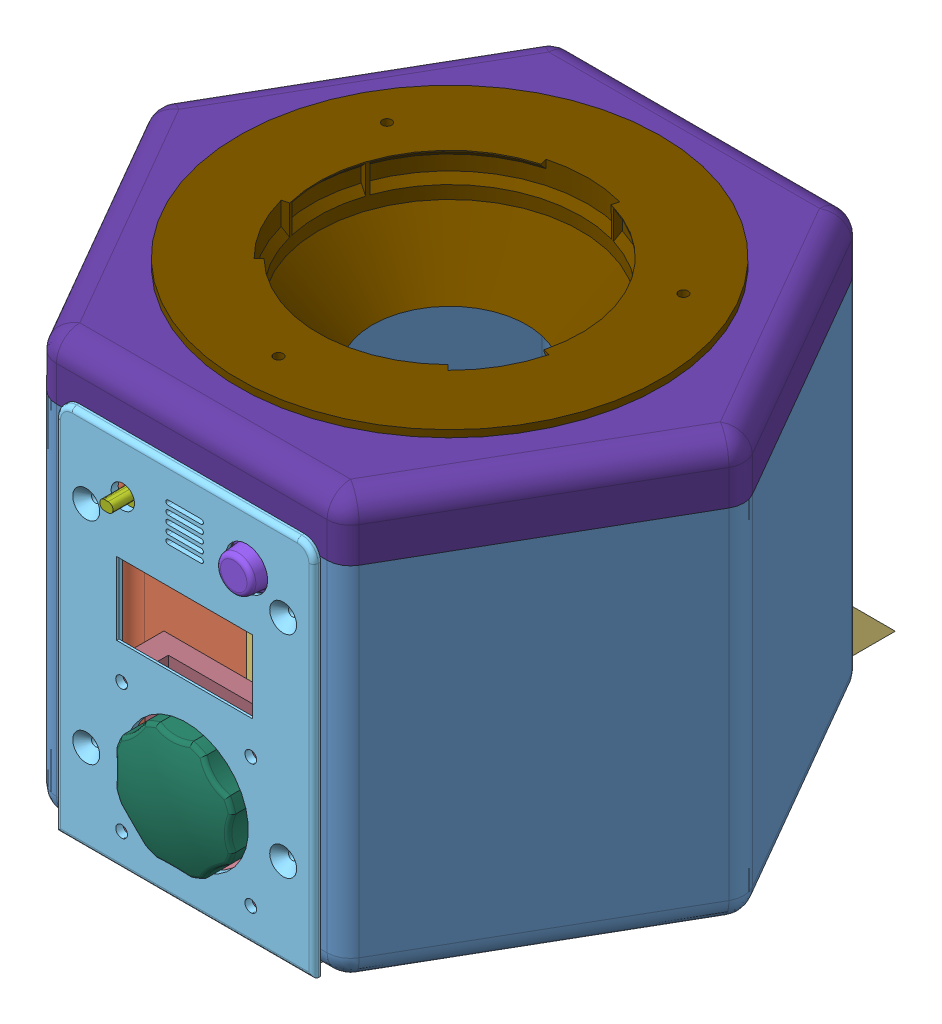
SolidWorks assembly Assy_base_tanque, configuration Default. Lengths in mm.
Overall size (250.94 210.12 285.79).
23 component instances, 18 part files, 9 mates.
Components (placement in the parent):
- base  1_1-1: base  1_1 [Default] at (121.3241 94.324 202.911) size (250.94 155 220)
- Assy_box_control-1: Assy_box_control [Default] at (251.8598 45.2792 -150.6249) size (110 187.12 285.79)
  - box-control_D-1: box-control_D [Default] at (-180.6357 49.0448 463.5359) size (50.1 155 250)
  - box-control_I-1: box-control_I [Default] at (-82.0357 49.0448 463.5359) size (50.1 155 250)
  - base_control_box-1: base_control_box [Default] at (-178.5357 49.0448 465.1037) size (96 25 220)
  - frente_control_box-1: frente_control_box [Default] at (-185.5357 49.0448 463.5359) size (110 160 8.5)
  - DS3231 RTC-2: DS3231 RTC [Default] at (-98.9357 55.5448 310.9359) x (0 0 -1) z (0 -1 0) size (44.75 22.8 13.53)
    - Default-1: Default [Predeterminado] at origin size (44.75 22.8 13.53)
  - LDR-1: LDR [Default] at (-156.876 173.9735 458.6019) x (1 0 0) z (0 0 -1) size (14.2 40.8 21.6)
  - MQ135_sensor-1: MQ135_sensor [Default] at (-98.6357 185.4448 458.0359) x (0 1 0) z (0 0 1) size (36.7 20 20.1)
  - ESP32_breadboard-1: ESP32_breadboard [Predeterminado] at (-142.2857 27.4234 204.8986) x (0 0 -1) z (1 0 0) size (186.74 40.42 55.48)
    - placa breadboard-1: placa breadboard [Predeterminado] at (-172.7373 28.1214 24.25) size (136 1.8 48.5)
    - 20-Pin Header - Female - 2.54mm-1: 20-Pin Header - Female - 2.54mm [Predeterminado] at (-93.0773 29.9214 11.43) size (51.3 8 2.5)
    - 20-Pin Header - Female - 2.54mm-2: 20-Pin Header - Female - 2.54mm [Predeterminado] at (-93.0773 29.9214 -11.43) size (51.3 8 2.5)
    - PCB_ESP32-38Pines-1: PCB_ESP32-38Pines [Predeterminado] at (-67.3173 36.9214 0) x (0 0 -1) z (1 0 0) size (28 10.12 55.48)
  - perilla-1: perilla [Predeterminado] at (-127.2204 86.8536 424.0509) size (65 65 36.44)
    - Rotary Encoder - KY-040-1: Rotary Encoder - KY-040 [Default] at (-4.2339 1.2762 17.985) size (19 30.75 32.39)
    - chasis_perilla-1: chasis_perilla [Predeterminado] at (-2.6839 3.7912 27.485) size (65 65 20.5)
    - rodamiento-1: rodamiento [Predeterminado] at (-2.6839 3.7912 33.485) x (1 0 0) z (0 -1 0) size (44.2 9 44.2)
    - perilla52-1: perilla52 [Predeterminado] at (-2.6839 3.7912 47.635) x (1 0 0) z (0 0 -1) size (52.46 52.46 20)
  - LoRa_Module_RA-02-1: LoRa_Module_RA-02 [Predeterminado] at (-94.5357 55.5448 278.6359) x (1 0 0) z (0 1 0) size (16 17 3.03)
- techo_tanque-1: techo_tanque [Predeterminado] at (121.3241 274.324 202.911) x (1 0 0) z (0 0 -1) size (250.94 30 220)
- embudo-1: embudo [Predeterminado] at (121.3241 277.324 202.911) x (0 -1 0) z (-0.5 0 0.866025) size (41.28 180 180)
Mates (geometry in assembly coordinates):
- Width1: width aligned: plane of base  1_1-1 through (70.3241 94.323 312.911) normal (1 0 0); plane of Assy_box_control-1/box-control_I-1 through (172.3241 94.323 312.911) normal (-1 0 0); plane of base  1_1-1 through (171.4241 94.324 312.911) normal (1 0 0); plane of Assy_box_control-1/box-control_D-1 through (71.2241 94.324 312.911) normal (-1 0 0)
- Coincident1: coincident anti-aligned: plane of base  1_1-1 through (57.8156 249.324 312.911) normal (0 0 1); plane of Assy_box_control-1/frente_control_box-1 through (73.3241 247.324 312.911) normal (0 0 -1)
- Coincident2: coincident anti-aligned: plane of base  1_1-1 through (70.3241 119.324 92.91) normal (0 -1 0); plane of Assy_box_control-1/box-control_D-1 through (72.8241 119.324 87.911) normal (0 1 0)
- Ancho1: width anti-aligned: plane of base  1_1-1 through (-5.693 249.324 202.911) normal (-0.866025 0 0.5); plane of techo_tanque-1 through (248.3411 249.324 202.911) normal (0.866025 0 -0.5); plane of base  1_1-1 through (184.8326 249.324 92.911) normal (0.866025 0 -0.5); plane of techo_tanque-1 through (57.8156 249.324 312.911) normal (-0.866025 0 0.5)
- Ancho2: width anti-aligned: plane of techo_tanque-1 through (-5.693 249.324 202.911) normal (-0.866025 0 -0.5); plane of base  1_1-1 through (248.3411 249.324 202.911) normal (0.866025 0 0.5); plane of techo_tanque-1 through (184.8326 249.324 312.911) normal (0.866025 0 0.5); plane of base  1_1-1 through (57.8156 249.324 92.911) normal (-0.866025 0 -0.5)
- Coincidente1: coincident anti-aligned: plane of base  1_1-1 through (121.3241 249.324 202.911) normal (0 1 0); plane of techo_tanque-1 through (121.3241 249.324 202.911) normal (0 -1 0)
- Concéntrica1: concentric anti-aligned: cylinder of techo_tanque-1 through (121.3241 274.325 202.911) axis (0 -1 0) radius 61; cylinder of embudo-1 through (121.3241 323.3579 202.911) axis (0 1 0) radius 60.1698
- Concéntrica2: concentric anti-aligned: cylinder of techo_tanque-1 through (58.1042 274.325 166.411) axis (0 -1 0) radius 2; cylinder of embudo-1 through (58.1042 272.324 166.411) axis (0 1 0) radius 2
- Coincidente2: coincident anti-aligned: plane of techo_tanque-1 through (121.3241 274.324 202.911) normal (0 1 0); plane of embudo-1 through (199.2664 274.324 247.911) normal (0 -1 0)
